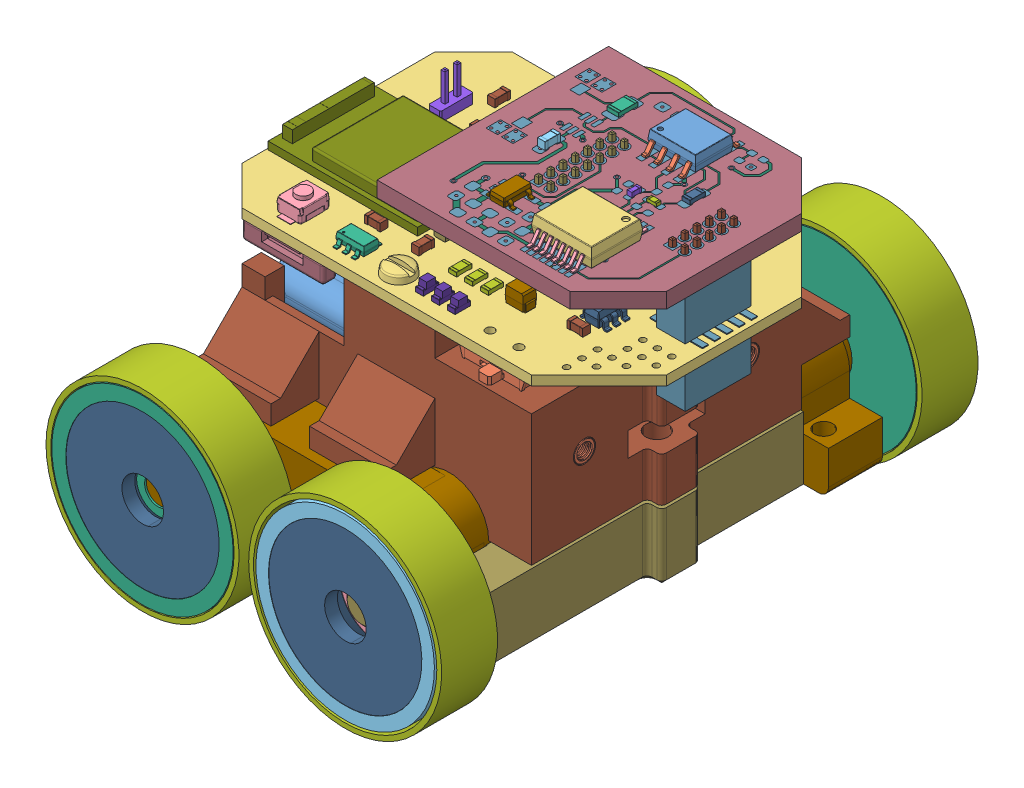
SolidWorks assembly AstroAnt_small_magnet, configuration Default. Lengths in mm.
Overall size (43.52 33.3 55.6).
182 component instances, 50 part files, 55 mates.
Components (placement in the parent):
- LiPo_360mAh-1: LiPo_360mAh [Default] at (6.0099 4.9998 47.0256) size (26.5 4.2 23.5) (hidden)
- 92120A150_Brass Heat-Set Inserts for Plastic-1: 92120A150_Brass Heat-Set Inserts for Plastic [92120A150] at (19.9543 12.4998 45.7029) size (2.56 3.33 2.56)
- 92120A150_Brass Heat-Set Inserts for Plastic-2: 92120A150_Brass Heat-Set Inserts for Plastic [92120A150] at (4.9543 12.4998 33.9529) size (2.56 3.33 2.56)
- 92120A150_Brass Heat-Set Inserts for Plastic-3: 92120A150_Brass Heat-Set Inserts for Plastic [92120A150] at (4.9543 12.4998 57.4529) size (2.56 3.33 2.56)
- 91460A005_METRIC CHEESE HEAD SLOTTED MACHINE SCREW-8: 91460A005_METRIC CHEESE HEAD SLOTTED MACHINE SCREW [91460A005] at (4.9543 14.9998 57.4529) x (1 0 0) z (0 1 0) size (3 3 7.1)
- 91460A005_METRIC CHEESE HEAD SLOTTED MACHINE SCREW-9: 91460A005_METRIC CHEESE HEAD SLOTTED MACHINE SCREW [91460A005] at (4.9543 14.9998 33.9529) x (1 0 0) z (0 1 0) size (3 3 7.1)
- 91460A005_METRIC CHEESE HEAD SLOTTED MACHINE SCREW-10: 91460A005_METRIC CHEESE HEAD SLOTTED MACHINE SCREW [91460A005] at (19.9543 14.9998 45.7029) x (1 0 0) z (0 1 0) size (3 3 7.1)
- 92120A150_Brass Heat-Set Inserts for Plastic-4: 92120A150_Brass Heat-Set Inserts for Plastic [92120A150] at (4.9543 -0.6002 57.4529) x (-0.616962 0 -0.786993) z (0.786993 0 -0.616962) size (2.56 3.33 2.56)
- 92120A150_Brass Heat-Set Inserts for Plastic-5: 92120A150_Brass Heat-Set Inserts for Plastic [92120A150] at (4.9543 -0.6002 33.9529) x (-0.616962 0 -0.786993) z (0.786993 0 -0.616962) size (2.56 3.33 2.56)
- mainboard_v1.step-1: mainboard_v1.step [Default] at (-103.0457 13.9998 235.7029) x (0 0 -1) z (0 1 0) size (29.41 41 10.8)
  - B3U-1000P.step-1: B3U-1000P.step [Default] at (178.95 -97.38 1.05) x (1 0 0) z (0 -1 0) size (4 1.75 2.5)
    - COMPOUND.step-1: COMPOUND.step [Default] at origin size (4 1.75 2.5)
  - 20021321-00014C1LF.step-1: 20021321-00014C1LF.step [Default] at (190 -115.5 1.05) size (9.35 5.45 4.85)
    - COMPOUND-0.step-1: COMPOUND-0.step [Default] at origin size (9.35 5.45 4.85)
  - MP6513GJ-Z.step-1: MP6513GJ-Z.step [Default] at (201.21 -120 1.05) x (-1 0 0) z (0 0 1) size (2.8 2.9 1)
    - COMPOUND-1.step-1: COMPOUND-1.step [Default] at origin size (2.8 2.9 1)
  - MP6513GJ-Z.step-2: MP6513GJ-Z.step [Default] at (178.51 -103.46 1.05) size (2.8 2.9 1)
    - COMPOUND-1.step-1: COMPOUND-1.step [Default] at origin size (2.8 2.9 1)
  - R_0603_1608Metric.step-1: R_0603_1608Metric.step [Default] at (195.55 -104.38 -0.05) x (1 0 0) z (0 0 -1) size (1.6 0.8 0.45)
    - SOLID.step-1: SOLID.step [Default] at origin size (1.6 0.8 0.45)
  - R_0603_1608Metric.step-2: R_0603_1608Metric.step [Default] at (192.6 -99.86 -0.05) x (0 1 0) z (0 0 -1) size (1.6 0.8 0.45)
    - SOLID.step-1: SOLID.step [Default] at origin size (1.6 0.8 0.45)
  - PinHeader_2x01_P1.27mm_Vertical.step-1: PinHeader_2x01_P1.27mm_Vertical.step [Default] at (194.96 -96.07 1.05) size (3.4 1.27 6.3)
    - SOLID-2.step-1: SOLID-2.step [Default] at origin size (3.4 1.27 6.3)
  - TAJP106K010RNJ.step-1: TAJP106K010RNJ.step [Default] at (196.22 -98.14 -0.05) x (-1 0 0) z (0 0 -1) size (2.05 1.4 1.7)
    - COMPOUND-3.step-1: COMPOUND-3.step [Default] at origin size (2.05 1.4 1.7)
  - TAJP106K010RNJ.step-2: TAJP106K010RNJ.step [Default] at (181.68 -117.23 1.05) x (0 1 0) z (0 0 1) size (2.05 1.4 1.7)
    - COMPOUND-3.step-1: COMPOUND-3.step [Default] at origin size (2.05 1.4 1.7)
  - SOT-23-5.step-1: SOT-23-5.step [Default] at (195.38 -122.78 1.05) x (0 1 0) z (0 0 1) size (2.8 2.9 1.55)
    - SOLID-4.step-1: SOLID-4.step [Default] at origin size (2.8 2.9 1.55)
  - C_0603_1608Metric.step-1: C_0603_1608Metric.step [Default] at (192.91 -122.55 1.05) x (0 -1 0) z (0 0 1) size (1.6 0.8 0.8)
    - SOLID-5.step-1: SOLID-5.step [Default] at origin size (1.6 0.8 0.8)
  - C_0603_1608Metric.step-2: C_0603_1608Metric.step [Default] at (193.57 -119.76 1.05) size (1.6 0.8 0.8)
    - SOLID-5.step-1: SOLID-5.step [Default] at origin size (1.6 0.8 0.8)
  - ECS-.327-12.5-12-TR.step-1: ECS-.327-12.5-12-TR.step [Default] at (184.31 -107.18 1.05) size (2 1.2 0.7)
    - COMPOUND-6.step-1: COMPOUND-6.step [Default] at origin size (2 1.2 0.7)
  - C_0603_1608Metric.step-3: C_0603_1608Metric.step [Default] at (197.67 -113.69 1.05) size (1.6 0.8 0.8)
    - SOLID-5.step-1: SOLID-5.step [Default] at origin size (1.6 0.8 0.8)
  - C_0603_1608Metric.step-4: C_0603_1608Metric.step [Default] at (197.64 -107.18 1.05) size (1.6 0.8 0.8)
    - SOLID-5.step-1: SOLID-5.step [Default] at origin size (1.6 0.8 0.8)
  - C_0603_1608Metric.step-5: C_0603_1608Metric.step [Default] at (190.96 -108.09 1.05) x (0 1 0) z (0 0 1) size (1.6 0.8 0.8)
    - SOLID-5.step-1: SOLID-5.step [Default] at origin size (1.6 0.8 0.8)
  - 1734592-6.step-1: 1734592-6.step [Default] at (203.79 -118 -1.05) x (0 -1 0) z (1 0 0) size (8.43 2.05 5.11)
    - SOLID-7.step-1: SOLID-7.step [Default] at origin size (8.43 2.05 5.11)
  - 1734592-6.step-2: 1734592-6.step [Default] at (176.19 -98 -1.05) x (0 1 0) z (-1 0 0) size (8.43 2.05 5.11)
    - SOLID-7.step-1: SOLID-7.step [Default] at origin size (8.43 2.05 5.11)
  - 20021321-00010C4LF.step-1: 20021321-00010C4LF.step [Default] at (190 -127.85 -0.05) x (1 0 0) z (0 0 -1) size (6.81 5.45 4.85)
    - COMPOUND-8.step-1: COMPOUND-8.step [Default] at origin size (6.81 5.45 4.85)
  - 20021321-00010C4LF.step-2: 20021321-00010C4LF.step [Default] at (190 -127.85 1.05) size (6.81 5.45 4.85)
    - COMPOUND-8.step-1: COMPOUND-8.step [Default] at origin size (6.81 5.45 4.85)
  - C_0603_1608Metric.step-6: C_0603_1608Metric.step [Default] at (181.31 -102.6 1.05) x (0 -1 0) z (0 0 1) size (1.6 0.8 0.8)
    - SOLID-5.step-1: SOLID-5.step [Default] at origin size (1.6 0.8 0.8)
  - C_0603_1608Metric.step-7: C_0603_1608Metric.step [Default] at (198.25 -119.14 1.05) x (0 -1 0) z (0 0 1) size (1.6 0.8 0.8)
    - SOLID-5.step-1: SOLID-5.step [Default] at origin size (1.6 0.8 0.8)
  - MPU6050.step-1: MPU6050.step [Default] at (198.43 -101.5 1.05) x (0 1 0) z (1 0 0) size (4 0.95 4)
    - COMPOUND-9.step-1: COMPOUND-9.step [Default] at origin size (4 0.95 4)
  - C_0603_1608Metric.step-8: C_0603_1608Metric.step [Default] at (194.9 -99.89 1.05) x (0 -1 0) z (0 0 1) size (1.6 0.8 0.8)
    - SOLID-5.step-1: SOLID-5.step [Default] at origin size (1.6 0.8 0.8)
  - C_0603_1608Metric.step-9: C_0603_1608Metric.step [Default] at (201.98 -100.38 1.05) x (0 -1 0) z (0 0 1) size (1.6 0.8 0.8)
    - SOLID-5.step-1: SOLID-5.step [Default] at origin size (1.6 0.8 0.8)
  - C_0603_1608Metric.step-10: C_0603_1608Metric.step [Default] at (201.98 -103.78 1.05) x (0 1 0) z (0 0 1) size (1.6 0.8 0.8)
    - SOLID-5.step-1: SOLID-5.step [Default] at origin size (1.6 0.8 0.8)
  - C_0603_1608Metric.step-11: C_0603_1608Metric.step [Default] at (198.81 -97.82 1.05) size (1.6 0.8 0.8)
    - SOLID-5.step-1: SOLID-5.step [Default] at origin size (1.6 0.8 0.8)
  - SOT-23-5.step-2: SOT-23-5.step [Default] at (184.86 -122.77 1.05) x (0 1 0) z (0 0 1) size (2.8 2.9 1.55)
    - SOLID-4.step-1: SOLID-4.step [Default] at origin size (2.8 2.9 1.55)
  - SOT-23-5.step-3: SOT-23-5.step [Default] at (197.58 -110.46 1.05) x (0 1 0) z (0 0 1) size (2.8 2.9 1.55)
    - SOLID-4.step-1: SOLID-4.step [Default] at origin size (2.8 2.9 1.55)
  - MDBT50Q-1MV2.step-1: MDBT50Q-1MV2.step [Default] at (187.3136 -98.605 1.0754) x (-1 0 0) z (0 1 0) size (10.5 2.06 15.5)
    - SOLID-10.step-1: SOLID-10.step [Default] at origin size (10.5 2.06 15.5)
  - C_0603_1608Metric.step-12: C_0603_1608Metric.step [Default] at (189.44 -108.09 1.05) x (0 1 0) z (0 0 1) size (1.6 0.8 0.8)
    - SOLID-5.step-1: SOLID-5.step [Default] at origin size (1.6 0.8 0.8)
  - C_0603_1608Metric.step-13: C_0603_1608Metric.step [Default] at (181.57 -107.18 1.05) x (-1 0 0) z (0 0 1) size (1.6 0.8 0.8)
    - SOLID-5.step-1: SOLID-5.step [Default] at origin size (1.6 0.8 0.8)
  - C_0603_1608Metric.step-14: C_0603_1608Metric.step [Default] at (186.97 -107.18 1.05) size (1.6 0.8 0.8)
    - SOLID-5.step-1: SOLID-5.step [Default] at origin size (1.6 0.8 0.8)
  - C_0603_1608Metric.step-15: C_0603_1608Metric.step [Default] at (184.77 -119.75 1.05) x (-1 0 0) z (0 0 1) size (1.6 0.8 0.8)
    - SOLID-5.step-1: SOLID-5.step [Default] at origin size (1.6 0.8 0.8)
  - C_0603_1608Metric.step-16: C_0603_1608Metric.step [Default] at (182.37 -122.54 1.05) x (0 -1 0) z (0 0 1) size (1.6 0.8 0.8)
    - SOLID-5.step-1: SOLID-5.step [Default] at origin size (1.6 0.8 0.8)
  - LED_0603_1608Metric.step-1: LED_0603_1608Metric.step [Default] at (178.19 -111.01 1.05) size (1.6 0.8 1.1)
    - SOLID-11.step-1: SOLID-11.step [Default] at origin size (1.6 0.8 1.1)
  - LED_0603_1608Metric.step-2: LED_0603_1608Metric.step [Default] at (178.19 -112.66 1.05) size (1.6 0.8 1.1)
    - SOLID-11.step-1: SOLID-11.step [Default] at origin size (1.6 0.8 1.1)
  - LED_0603_1608Metric.step-3: LED_0603_1608Metric.step [Default] at (178.19 -114.31 1.05) size (1.6 0.8 1.1)
    - SOLID-11.step-1: SOLID-11.step [Default] at origin size (1.6 0.8 1.1)
  - LED_0603_1608Metric.step-4: LED_0603_1608Metric.step [Default] at (202.34 -112.21 1.05) x (0 1 0) z (0 0 1) size (1.6 0.8 1.1)
    - SOLID-11.step-1: SOLID-11.step [Default] at origin size (1.6 0.8 1.1)
  - 473460001.step-1: 473460001.step [Default] at (201.68 -99.72 -1.25) x (0 -1 0) z (1 0 0) size (7.98 2.94 5.43)
    - COMPOUND-12.step-1: COMPOUND-12.step [Default] at origin size (7.98 2.94 5.43)
  - L_0603_1608Metric.step-1: L_0603_1608Metric.step [Default] at (192.48 -108.09 1.05) x (0 1 0) z (0 0 1) size (1.6 0.8 0.8)
    - SOLID-13.step-1: SOLID-13.step [Default] at origin size (1.6 0.8 0.8)
  - R_0603_1608Metric.step-3: R_0603_1608Metric.step [Default] at (185.18 -111.31 1.05) x (-1 0 0) z (0 0 1) size (1.6 0.8 0.45)
    - SOLID.step-1: SOLID.step [Default] at origin size (1.6 0.8 0.45)
  - R_0603_1608Metric.step-4: R_0603_1608Metric.step [Default] at (185.18 -109.77 1.05) size (1.6 0.8 0.45)
    - SOLID.step-1: SOLID.step [Default] at origin size (1.6 0.8 0.45)
  - R_0603_1608Metric.step-5: R_0603_1608Metric.step [Default] at (181.62 -111.01 1.05) size (1.6 0.8 0.45)
    - SOLID.step-1: SOLID.step [Default] at origin size (1.6 0.8 0.45)
  - R_0603_1608Metric.step-6: R_0603_1608Metric.step [Default] at (181.62 -112.66 1.05) size (1.6 0.8 0.45)
    - SOLID.step-1: SOLID.step [Default] at origin size (1.6 0.8 0.45)
  - R_0603_1608Metric.step-7: R_0603_1608Metric.step [Default] at (181.62 -114.31 1.05) x (-1 0 0) z (0 0 1) size (1.6 0.8 0.45)
    - SOLID.step-1: SOLID.step [Default] at origin size (1.6 0.8 0.45)
  - R_0603_1608Metric.step-8: R_0603_1608Metric.step [Default] at (194.84 -108.1 1.05) x (0 1 0) z (0 0 1) size (1.6 0.8 0.45)
    - SOLID.step-1: SOLID.step [Default] at origin size (1.6 0.8 0.45)
  - R_0603_1608Metric.step-9: R_0603_1608Metric.step [Default] at (200.69 -112.2325 1.05) x (0 1 0) z (0 0 1) size (1.6 0.8 0.45)
    - SOLID.step-1: SOLID.step [Default] at origin size (1.6 0.8 0.45)
  - R_0603_1608Metric.step-10: R_0603_1608Metric.step [Default] at (196.22 -101.51 -0.05) x (-1 0 0) z (0 0 -1) size (1.6 0.8 0.45)
    - SOLID.step-1: SOLID.step [Default] at origin size (1.6 0.8 0.45)
  - R_0603_1608Metric.step-11: R_0603_1608Metric.step [Default] at (196.22 -99.9725 -0.05) x (-1 0 0) z (0 0 -1) size (1.6 0.8 0.45)
    - SOLID.step-1: SOLID.step [Default] at origin size (1.6 0.8 0.45)
  - SW_SPDT_PCM12.step-1: SW_SPDT_PCM12.step [Default] at (178.18 -119.37 -0.05) x (0 1 0) z (0 0 -1) size (7.7 5 2)
    - SOLID-14.step-1: SOLID-14.step [Default] at origin size (7.7 5 2)
  - COMPOUND-15.step-1: COMPOUND-15.step [Default] at origin size (28 41 1)
- ball_bearing_5x11x4mm-1: ball_bearing_5x11x4mm [Default] at (-65.9801 -4.7758 21.2029) x (0.999925 -0.012245 0) z (0 0 1) size (8 8 2.5)
- wheel_holder_non_motor-1: wheel_holder_non_motor [Default] at (-90.7699 -0.8362 17.9029) size (18.5 18.5 5.8)
- wheel_holder_non_motor-2: wheel_holder_non_motor [Default] at (1.3792 -86.6559 73.5029) x (0.185441 0.982655 0) z (0 0 -1) size (18.5 18.5 5.8)
- ball_bearing_5x11x4mm-2: ball_bearing_5x11x4mm [Default] at (-9.788 -57.5376 70.2029) x (0.373101 0.927791 0) z (0 0 -1) size (8 8 2.5)
- wheel_motor-1: wheel_motor [Default] at (44.5289 -0.8963 17.9029) size (18.8 18.8 5.8)
- wheel_motor-2: wheel_motor [Default] at (-4.9746 26.526 73.5029) x (-0.038296 0.999266 0) z (0 0 -1) size (18.8 18.8 5.8)
- tire-1: tire [Default] at (58.6593 -4.042 17.9029) size (20 20 5.8)
- tire-2: tire [Default] at (37.6493 -4.042 17.9029) size (20 20 5.8)
- tire-3: tire [Default] at (58.6593 -4.042 67.7029) size (20 20 5.8)
- tire-4: tire [Default] at (37.6493 -4.042 67.7029) size (20 20 5.8)
- PA2-50_with_gearbox-3: PA2-50_with_gearbox [Default] at (45.51 -3.6027 60.1029) x (-1 0 0) z (0 0 1) size (30.92 12.52 38.5)
  - PA2-50-1: PA2-50 [Default] at (26.117 -19.7771 -19.1) x (0 0 1) z (0.954024 0.299729 0) size (29.1 8 8) (hidden)
  - gearbox-1: gearbox [Default] at origin size (29.9 11.5 13.6)
- PA2-50_with_gearbox-4: PA2-50_with_gearbox [Default] at (-35.6268 -3.6027 31.3029) x (1 0 0) z (0 0 -1) size (30.92 12.52 38.5)
  - PA2-50-1: PA2-50 [Default] at (26.117 -19.7771 -19.1) x (0 0 1) z (0.954024 0.299729 0) size (29.1 8 8) (hidden)
  - gearbox-1: gearbox [Default] at origin size (29.9 11.5 13.6)
- RA22CS-N-1: RA22CS-N [Default] at (15.4466 -2.6002 19.5154) x (1 0 0) z (0 -1 0) size (15.88 3.17 15.88)
- RA22CS-N-2: RA22CS-N [Default] at (-5.5634 -2.6002 19.5154) x (1 0 0) z (0 -1 0) size (15.88 3.17 15.88)
- RA22CS-N-3: RA22CS-N [Default] at (-5.5634 -2.6002 71.8904) x (-0.968047 -0.250767 0) z (0.250767 -0.968047 0) size (15.88 3.17 15.88)
- RA22CS-N-4: RA22CS-N [Default] at (15.4466 -2.6002 71.8904) x (-0.968047 -0.250767 0) z (0.250767 -0.968047 0) size (15.88 3.17 15.88)
- robobody-1: robobody [Default] at (-9.0457 6.9406 -0.9986) size (31.5 16.1 38)
- 92120A150_Brass Heat-Set Inserts for Plastic-6: 92120A150_Brass Heat-Set Inserts for Plastic [92120A150] at (19.9543 -0.6002 45.7029) x (-0.616962 0 -0.786993) z (0.786993 0 -0.616962) size (2.56 3.33 2.56)
- motor_holder_2-1: motor_holder_2 [Default] at (52.4112 -9.4002 -5.2676) size (31.5 8.8 52.2)
- 92120A150_Brass Heat-Set Inserts for Plastic-7: 92120A150_Brass Heat-Set Inserts for Plastic [92120A150] at (19.4543 5.3998 54.2029) x (0 1 0) z (0 0 1) size (2.56 3.33 2.56)
- 92120A150_Brass Heat-Set Inserts for Plastic-8: 92120A150_Brass Heat-Set Inserts for Plastic [92120A150] at (19.4543 5.3998 37.2029) x (0 1 0) z (0 0 1) size (2.56 3.33 2.56)
- impedance_measurement2-impedance_measurement.step-1: impedance_measurement2-impedance_measurement.step [Default] at (27.9543 22.4998 52.7029) x (0 0 -1) z (0 1 0) size (24 25 7.6) (hidden)
  - Board_Geoms_58a9.step-1: Board_Geoms_58a9.step [Default] at origin size (24 25 1.65)
    - Pcb_58a9.step-1: Pcb_58a9.step [Default] at (-125 125 0) size (24 25 1.6)
    - topPads_58a9.step-1: topPads_58a9.step [Default] at (-125 125 0.02) size (21.67 21.95 0.01)
    - topTracks_58a9.step-1: topTracks_58a9.step [Default] at (-125 125 0.01) size (22.19 20.2 0.01)
    - topZones_58a9.step-1: topZones_58a9.step [Default] at (-125 125 0.01) size (1.81 1.01 0.01)
    - botPads_58a9.step-1: botPads_58a9.step [Default] at (-125 125 -1.62) size (20.66 21.93 0.01)
    - botTracks_58a9.step-1: botTracks_58a9.step [Default] at (-125 125 -1.61) size (19.15 19.69 0.01)
    - botZones_58a9.step-1: botZones_58a9.step [Default] at (-125 125 -1.61)
  - Step_Models_58a9.step-1: Step_Models_58a9.step [Default] at origin size (21.21 18.41 7.6)
    - Top_58a9.step-1: Top_58a9.step [Default] at origin size (21.21 14.13 2)
      - U1_ASSEMBLY_616EAA5E.step-1: U1_ASSEMBLY_616EAA5E.step [Default] at (13.84 11.34 0) size (6 4.9 1.75)
        - Body.step-1: Body.step [Default] at origin size (3.9 4.9 1.57)
        - PinsArrayLR.step-1: PinsArrayLR.step [Default] at origin size (6 4.22 1)
      - U2_ASSEMBLY_6195A977.step-1: U2_ASSEMBLY_6195A977.step [Default] at (0.61 8.84 0) x (-1 0 0) z (0 0 1) size (7.8 6.2 2)
        - Body001.step-1: Body001.step [Default] at origin size (5.3 6.2 1.95)
        - PinsArrayLR001.step-1: PinsArrayLR001.step [Default] at origin size (7.8 4.85 1.09)
      - C9_C_0603_1608Metric_6195A5CF.step-1: C9_C_0603_1608Metric_6195A5CF.step [Default] at (7.13 19.31 0) size (1.6 0.8 0.8)
      - R11_R_0805_2012Metric_6195A804.step-1: R11_R_0805_2012Metric_6195A804.step [Default] at (14.1 18.66 0) size (2 1.2 0.45)
      - C9_C_0603_1608Metric_6195A5CF.step-2: C9_C_0603_1608Metric_6195A5CF.step [Default] at (16.32 15.88 0) x (0 -1 0) z (0 0 1) size (1.6 0.8 0.8)
      - R10_R_0402_1005Metric_inf.step-1: R10_R_0402_1005Metric_inf.step [Default] at (7.27 8.57 0) x (0 1 0) z (0 0 1) size (1 0.5 0.35)
      - R10_R_0402_1005Metric_inf.step-2: R10_R_0402_1005Metric_inf.step [Default] at (6.06 8.57 0) x (0 1 0) z (0 0 1) size (1 0.5 0.35)
      - R10_R_0402_1005Metric_inf.step-3: R10_R_0402_1005Metric_inf.step [Default] at (9.01 9.43 0) x (-1 0 0) z (0 0 1) size (1 0.5 0.35)
      - R10_R_0402_1005Metric_inf.step-4: R10_R_0402_1005Metric_inf.step [Default] at (7.06 11.59 0) x (-1 0 0) z (0 0 1) size (1 0.5 0.35)
      - R10_R_0402_1005Metric_inf.step-5: R10_R_0402_1005Metric_inf.step [Default] at (15.52 7.36 0) x (0 1 0) z (0 0 1) size (1 0.5 0.35)
      - R10_R_0402_1005Metric_inf.step-6: R10_R_0402_1005Metric_inf.step [Default] at (16.82 7.36 0) x (0 -1 0) z (0 0 1) size (1 0.5 0.35)
      - C5_C_0402_1005Metric_616E5CDC.step-1: C5_C_0402_1005Metric_616E5CDC.step [Default] at (7.09 10.42 0) x (-1 0 0) z (0 0 1) size (1 0.5 0.5)
      - U3_TSOT_23_5_616E36B3.step-1: U3_TSOT_23_5_616E36B3.step [Default] at (0.38 16.55 0) x (0 -1 0) z (0 0 1) size (2.8 2.9 0.95)
      - R8_R_0603_1608Metric_inf.step-1: R8_R_0603_1608Metric_inf.step [Default] at (9.74 6.91 0) x (-1 0 0) z (0 0 1) size (1.6 0.8 0.45)
      - C9_C_0603_1608Metric_6195A5CF.step-3: C9_C_0603_1608Metric_6195A5CF.step [Default] at (-2.15 17 0) x (0 1 0) z (0 0 1) size (1.6 0.8 0.8)
      - C9_C_0603_1608Metric_6195A5CF.step-4: C9_C_0603_1608Metric_6195A5CF.step [Default] at (0.46 13.71 0) size (1.6 0.8 0.8)
      - C9_C_0603_1608Metric_6195A5CF.step-5: C9_C_0603_1608Metric_6195A5CF.step [Default] at (-1.47 19.47 0) size (1.6 0.8 0.8)
      - C9_C_0603_1608Metric_6195A5CF.step-6: C9_C_0603_1608Metric_6195A5CF.step [Default] at (-2.96 12.84 0) size (1.6 0.8 0.8)
      - C9_C_0603_1608Metric_6195A5CF.step-7: C9_C_0603_1608Metric_6195A5CF.step [Default] at (-3.74 17.02 0) x (0 -1 0) z (0 0 1) size (1.6 0.8 0.8)
      - C9_C_0603_1608Metric_6195A5CF.step-8: C9_C_0603_1608Metric_6195A5CF.step [Default] at (-2.96 14.45 0) x (-1 0 0) z (0 0 1) size (1.6 0.8 0.8)
    - Bot_58a9.step-1: Bot_58a9.step [Default] at origin size (14.64 18.41 6.3)
      - R10_R_0402_1005Metric_inf.step-1: R10_R_0402_1005Metric_inf.step [Default] at (-2.7 9.16 -1.6) x (-1 0 0) z (0 0 -1) size (1 0.5 0.35)
      - R10_R_0402_1005Metric_inf.step-2: R10_R_0402_1005Metric_inf.step [Default] at (3.08 7.15 -1.6) x (1 0 0) z (0 0 -1) size (1 0.5 0.35)
      - R10_R_0402_1005Metric_inf.step-3: R10_R_0402_1005Metric_inf.step [Default] at (1.08 9.94 -1.6) x (-0.707107 -0.707107 0) z (0 0 -1) size (1 0.5 0.35)
      - J4_PinHeader_2x05_P127mm_Vertical_616E426E.step-1: J4_PinHeader_2x05_P127mm_Vertical_616E426E.step [Default] at (4.46 3.83 -1.6) x (0 -1 0) z (0 0 -1) size (3.4 6.35 6.3)
      - J3_PinHeader_2x07_P127mm_Vertical_616E4D18.step-1: J3_PinHeader_2x07_P127mm_Vertical_616E4D18.step [Default] at (3.19 16.45 -1.6) x (0 -1 0) z (0 0 -1) size (3.4 8.89 6.3)
      - C9_C_0603_1608Metric_6195A5CF.step-1: C9_C_0603_1608Metric_6195A5CF.step [Default] at (2.85 19.51 -1.6) x (-1 0 0) z (0 0 -1) size (1.6 0.8 0.8)
- 9mm_pogo_pin-1: 9mm_pogo_pin [Default] at (4.8543 -7.1002 37.7029) x (0.948575 0 -0.316551) z (0.316551 0 0.948575) size (2 9 2) (hidden)
- 9mm_pogo_pin-2: 9mm_pogo_pin [Default] at (4.8543 -7.1002 53.7029) x (0.905311 0 -0.424749) z (0.424749 0 0.905311) size (2 9 2) (hidden)
Mates (geometry in assembly coordinates):
- Concentric63: concentric anti-aligned: cylinder of ball_bearing_5x11x4mm-1 through (-5.5634 -2.6002 23.7029) axis (0 0 -1) radius 4; cylinder of wheel_holder_non_motor-1 through (-5.5634 -2.6002 17.9029) axis (0 0 1) radius 4
- Coincident105: coincident aligned: plane of ball_bearing_5x11x4mm-1 through (-5.5634 -2.6002 23.7029) normal (0 0 1); plane of wheel_holder_non_motor-1 through (-5.5634 -2.6002 23.7029) normal (0 0 1)
- Coincident107: coincident aligned: plane of wheel_holder_non_motor-2 through (15.4466 -2.6002 67.7029) normal (0 0 -1); plane of ball_bearing_5x11x4mm-2 through (15.4466 -2.6002 67.7029) normal (0 0 -1)
- Concentric83: concentric anti-aligned: cylinder of wheel_motor-1 through (15.4466 -2.6002 23.7029) axis (0 0 -1) radius 9.4; cylinder of tire-1 through (15.4466 -2.6002 17.9029) axis (0 0 1) radius 9.5
- Coincident123: coincident aligned: plane of wheel_motor-1 through (15.4466 -2.6002 17.9029) normal (0 0 -1); plane of tire-1 through (15.4466 -2.6002 17.9029) normal (0 0 -1)
- Concentric84: concentric anti-aligned: cylinder of wheel_holder_non_motor-1 through (-5.5634 -2.6002 23.7029) axis (0 0 -1) radius 9.25; cylinder of tire-2 through (-5.5634 -2.6002 17.9029) axis (0 0 1) radius 9.5
- Coincident124: coincident aligned: plane of wheel_holder_non_motor-1 through (-5.5634 -2.6002 17.9029) normal (0 0 -1); plane of tire-2 through (-5.5634 -2.6002 17.9029) normal (0 0 -1)
- Coincident125: coincident aligned: plane of wheel_motor-2 through (-5.5634 -2.6002 73.5029) normal (0 0 1); plane of tire-4 through (-5.5634 -2.6002 73.5029) normal (0 0 1)
- Concentric85: concentric aligned: cylinder of wheel_motor-2 through (-5.5634 -2.6002 67.7029) axis (0 0 1) radius 9.4; cylinder of tire-4 through (-5.5634 -2.6002 67.7029) axis (0 0 1) radius 9.5
- Coincident126: coincident aligned: plane of wheel_holder_non_motor-2 through (15.4466 -2.6002 73.5029) normal (0 0 1); plane of tire-3 through (15.4466 -2.6002 73.5029) normal (0 0 1)
- Concentric86: concentric aligned: cylinder of wheel_holder_non_motor-2 through (15.4466 -2.6002 67.7029) axis (0 0 1) radius 9.25; cylinder of tire-3 through (15.4466 -2.6002 67.7029) axis (0 0 1) radius 9.5
- Concentric100: concentric anti-aligned: cylinder of wheel_holder_non_motor-2 through (15.4466 -2.6002 73.5029) axis (0 0 -1) radius 4; cylinder of ball_bearing_5x11x4mm-2 through (15.4466 -2.6002 66.2029) axis (0 0 1) radius 2
- Coincident138: coincident aligned: plane of wheel_holder_non_motor-2 through (15.4466 -2.6002 67.7029) normal (0 0 -1); plane of ball_bearing_5x11x4mm-2 through (15.4466 -2.6002 67.7029) normal (0 0 -1)
- Concentric110: concentric anti-aligned: cylinder of wheel_motor-2 through (-5.5634 -2.6002 67.7029) axis (0 0 1) radius 1.4; cylinder of PA2-50_with_gearbox-3/gearbox-1 through (-5.5634 -2.6002 71.7029) axis (0 0 -1) radius 1.45
- Concentric111: concentric aligned: cylinder of tire-1 through (15.4466 -2.6002 23.7029) axis (0 0 -1) radius 10; cylinder of tire-3 through (15.4466 -2.6002 73.5029) axis (0 0 -1) radius 10
- Concentric112: concentric aligned: cylinder of tire-2 through (-5.5634 -2.6002 23.7029) axis (0 0 -1) radius 10; cylinder of tire-4 through (-5.5634 -2.6002 73.5029) axis (0 0 -1) radius 10
- Coincident144: coincident aligned: plane of PA2-50_with_gearbox-3/gearbox-1 through (16.4366 -9.1002 65.7029) normal (0 -1 0); plane of PA2-50_with_gearbox-4/gearbox-1 through (-6.5534 -9.1002 25.7029) normal (0 -1 0)
- Coincident145: coincident aligned: plane of wheel_holder_non_motor-1 through (-5.5634 -2.6002 17.9029) normal (0 0 -1); plane of wheel_motor-1 through (15.4466 -2.6002 17.9029) normal (0 0 -1)
- Coincident146: coincident aligned: plane of wheel_holder_non_motor-2 through (15.4466 -2.6002 73.5029) normal (0 0 1); plane of wheel_motor-2 through (-5.5634 -2.6002 73.5029) normal (0 0 1)
- Coincident149: coincident anti-aligned: plane of wheel_motor-1 through (15.4466 -2.6002 21.1029) normal (0 0 -1); plane of RA22CS-N-1 through (15.4466 -2.6002 21.1029) normal (0 0 1)
- Concentric113: concentric aligned: cylinder of wheel_motor-1 through (15.4466 -2.6002 23.7029) axis (0 0 -1) radius 1.4; cylinder of RA22CS-N-1 through (15.4466 -2.6002 19.5154) axis (0 0 -1) radius 2.159
- Concentric114: concentric aligned: cylinder of wheel_holder_non_motor-1 through (-5.5634 -2.6002 21.1029) axis (0 0 -1) radius 7.95; cylinder of RA22CS-N-2 through (-5.5634 -2.6002 19.5154) axis (0 0 -1) radius 2.159
- Coincident150: coincident anti-aligned: plane of wheel_holder_non_motor-1 through (-5.5634 -2.6002 21.1029) normal (0 0 -1); plane of RA22CS-N-2 through (-5.5634 -2.6002 21.1029) normal (0 0 1)
- Concentric115: concentric aligned: cylinder of wheel_motor-2 through (-5.5634 -2.6002 70.3029) axis (0 0 1) radius 7.95; cylinder of RA22CS-N-3 through (-5.5634 -2.6002 70.3029) axis (0 0 1) radius 7.9375
- Coincident151: coincident anti-aligned: plane of wheel_motor-2 through (-5.5634 -2.6002 70.3029) normal (0 0 1); plane of RA22CS-N-3 through (-5.5634 -2.6002 70.3029) normal (0 0 -1)
- Concentric116: concentric aligned: cylinder of wheel_holder_non_motor-2 through (15.4466 -2.6002 70.3029) axis (0 0 1) radius 7.95; cylinder of RA22CS-N-4 through (15.4466 -2.6002 70.3029) axis (0 0 1) radius 7.9375
- Coincident152: coincident anti-aligned: plane of wheel_holder_non_motor-2 through (15.4466 -2.6002 70.3029) normal (0 0 1); plane of RA22CS-N-4 through (15.4466 -2.6002 70.3029) normal (0 0 -1)
- Coincident153: coincident aligned: plane of mainboard_v1.step-1/COMPOUND-15.step-1 through (20.9543 13.9998 59.7029) normal (0 0 1); plane of robobody-1 through (20.9543 13.9998 59.7029) normal (0 0 1)
- Coincident154: coincident: line of mainboard_v1.step-1/COMPOUND-15.step-1 through (-9.0457 13.9998 59.7029) axis (0 1 0); plane of robobody-1 through (-9.0457 6.9406 -0.9986) normal (-1 0 0)
- Concentric121: concentric aligned: cylinder of 92120A150_Brass Heat-Set Inserts for Plastic-4 through (4.9543 0.8998 57.4529) axis (0 1 0) radius 1.075; cylinder of robobody-1 through (4.9543 -2.1591 57.4529) axis (0 1 0) radius 1.15
- Concentric122: concentric aligned: cylinder of 92120A150_Brass Heat-Set Inserts for Plastic-5 through (4.9543 0.8998 33.9529) axis (0 1 0) radius 1.075; cylinder of robobody-1 through (4.9543 -2.1591 33.9529) axis (0 1 0) radius 1.15
- Concentric123: concentric aligned: cylinder of robobody-1 through (19.9543 -2.1591 45.7029) axis (0 1 0) radius 1.15; cylinder of 92120A150_Brass Heat-Set Inserts for Plastic-6 through (19.9543 0.8998 45.7029) axis (0 1 0) radius 1.075
- Coincident164: coincident anti-aligned: plane of PA2-50_with_gearbox-4/gearbox-1 through (12.2966 -5.4002 30.3029) normal (0 -1 0); plane of motor_holder_2-1 through (-9.0457 -5.4002 31.5029) normal (0 1 0)
- Coincident167: coincident aligned: plane of robobody-1 through (20.9543 6.9406 -0.9986) normal (1 0 0); plane of motor_holder_2-1 through (20.9543 -2.4002 61.1029) normal (1 0 0)
- Concentric124: concentric anti-aligned: cylinder of PA2-50_with_gearbox-3/PA2-50-1 through (12.4366 -2.1002 57.2029) axis (0 0 -1) radius 4; cylinder of robobody-1 through (12.4366 -2.1002 32.5029) axis (0 0 1) radius 4.1
- Concentric125: concentric anti-aligned: cylinder of PA2-50_with_gearbox-4/PA2-50-1 through (-2.5534 -2.1002 34.2029) axis (0 0 1) radius 4; cylinder of robobody-1 through (-2.5534 -2.1002 58.9029) axis (0 0 -1) radius 4.1
- Coincident174: coincident anti-aligned: plane of PA2-50_with_gearbox-4/gearbox-1 through (-2.5534 -2.1002 31.7029) normal (0 0 1); plane of robobody-1 through (20.9543 13.9998 31.7029) normal (0 0 -1)
- Coincident175: coincident anti-aligned: plane of PA2-50_with_gearbox-3/gearbox-1 through (12.4366 -2.1002 59.7029) normal (0 0 -1); plane of robobody-1 through (20.9543 13.9998 59.7029) normal (0 0 1)
- Coincident176: coincident anti-aligned: plane of mainboard_v1.step-1/COMPOUND-15.step-1 through (6.7692 13.9998 45.7029) normal (0 -1 0); plane of robobody-1 through (20.9543 13.9998 59.7029) normal (0 1 0)
- Concentric126: concentric anti-aligned: cylinder of robobody-1 through (14.5016 5.3998 54.2029) axis (1 0 0) radius 1.15; cylinder of 92120A150_Brass Heat-Set Inserts for Plastic-7 through (17.9543 5.3998 54.2029) axis (-1 0 0) radius 1.075
- Concentric127: concentric anti-aligned: cylinder of robobody-1 through (14.5016 5.3998 37.2029) axis (1 0 0) radius 1.15; cylinder of 92120A150_Brass Heat-Set Inserts for Plastic-8 through (17.9543 5.3998 37.2029) axis (-1 0 0) radius 1.075
- Coincident177: coincident aligned: plane of robobody-1 through (20.9543 6.9406 -0.9986) normal (1 0 0); plane of 92120A150_Brass Heat-Set Inserts for Plastic-8 through (20.9543 4.5998 37.2029) normal (1 0 0)
- Coincident178: coincident aligned: plane of robobody-1 through (20.9543 6.9406 -0.9986) normal (1 0 0); plane of 92120A150_Brass Heat-Set Inserts for Plastic-7 through (20.9543 4.5998 54.2029) normal (1 0 0)
- Distance1: distance = 2 mm anti-aligned: plane of wheel_motor-2 through (-5.5634 -2.6002 67.7029) normal (0 0 -1); plane of PA2-50_with_gearbox-3/gearbox-1 through (45.51 -3.6027 65.7029) normal (0 0 1)
- Distance2: distance = 2 mm anti-aligned: plane of wheel_motor-1 through (15.4466 -2.6002 23.7029) normal (0 0 1); plane of PA2-50_with_gearbox-4/gearbox-1 through (-35.6268 -3.6027 25.7029) normal (0 0 -1)
- Concentric128: concentric anti-aligned: cylinder of PA2-50_with_gearbox-4/gearbox-1 through (15.4466 -2.6002 19.7029) axis (0 0 1) radius 1.45; cylinder of RA22CS-N-1 through (15.4466 -2.6002 19.5154) axis (0 0 -1) radius 2.159
- Distance9: distance = 0.25 mm anti-aligned: plane of LiPo_360mAh-1 through (15.7543 9.1998 57.4529) normal (0 0 1); plane of robobody-1 through (42.4929 9.9998 57.7029) normal (0 0 -1)
- Coincident222: coincident anti-aligned: plane of LiPo_360mAh-1 through (17.7543 4.9998 47.0256) normal (1 0 0); plane of robobody-1 through (17.7543 3.9998 36.2029) normal (-1 0 0)
- Coincident223: coincident anti-aligned: plane of mainboard_v1.step-1/20021321-00010C4LF.step-2/COMPOUND-8.step-1 through (24.8043 19.8998 45.7029) normal (0 1 0); plane of impedance_measurement2-impedance_measurement.step-1/Step_Models_58a9.step-1/Bot_58a9.step-1/J4_PinHeader_2x05_P127mm_Vertical_616E426E.step-1 through (24.7593 19.8998 45.7029) normal (0 -1 0)
- Coincident224: coincident aligned: plane of mainboard_v1.step-1/COMPOUND-15.step-1 through (27.9543 13.9998 38.7029) normal (1 0 0); plane of impedance_measurement2-impedance_measurement.step-1/Board_Geoms_58a9.step-1/Pcb_58a9.step-1 through (27.9543 22.4998 38.7029) normal (1 0 0)
- Distance10: distance = 0.23 mm aligned: plane of impedance_measurement2-impedance_measurement.step-1/Step_Models_58a9.step-1/Bot_58a9.step-1/J4_PinHeader_2x05_P127mm_Vertical_616E426E.step-1 through (23.1863 20.8998 42.5279) normal (0 0 -1); plane of mainboard_v1.step-1/20021321-00010C4LF.step-2/COMPOUND-8.step-1 through (23.3043 15.1498 42.2979) normal (0 0 -1)
- Concentric129: concentric anti-aligned: cylinder of robobody-1 through (4.8543 -7.2616 53.7029) axis (0 -1 0) radius 1.5; cylinder of 9mm_pogo_pin-2 through (4.8543 -11.6002 53.7029) axis (0 1 0) radius 0.75
- Concentric130: concentric anti-aligned: cylinder of robobody-1 through (4.8543 -7.2616 37.7029) axis (0 -1 0) radius 1.5; cylinder of 9mm_pogo_pin-1 through (4.8543 -11.6002 37.7029) axis (0 1 0) radius 0.75
- Distance11: distance = 4.2 mm aligned: plane of 9mm_pogo_pin-2 through (4.8543 -13.6002 53.7029) normal (0 -1 0); plane of motor_holder_2-1 through (52.4112 -9.4002 -5.2676) normal (0 -1 0)
- Distance12: distance = 4.2 mm aligned: plane of 9mm_pogo_pin-1 through (4.8543 -13.6002 37.7029) normal (0 -1 0); plane of motor_holder_2-1 through (52.4112 -9.4002 -5.2676) normal (0 -1 0)
